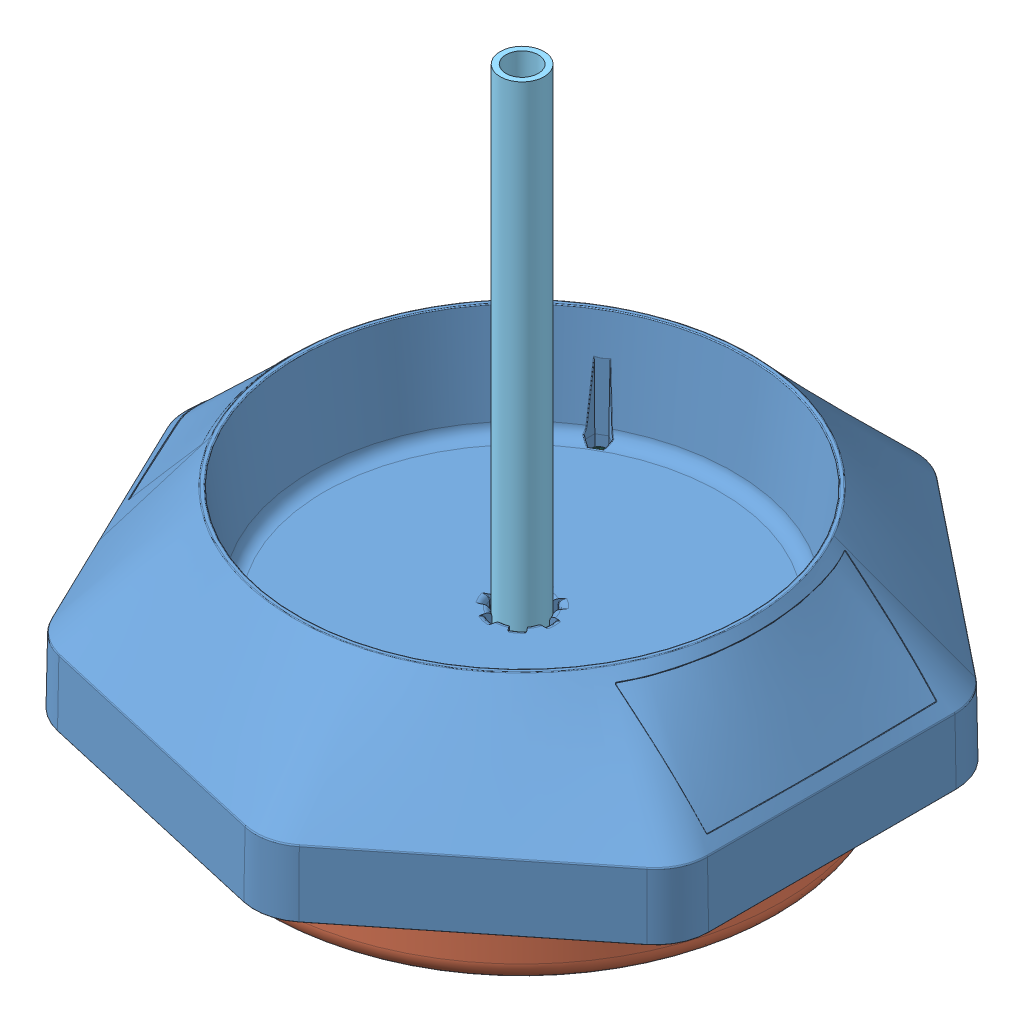
SolidWorks assembly BlueMogo, configuration Default. Lengths in mm.
Overall size (329.62 312.25 329.62).
18 component instances, 8 part files, 0 mates.
Components (placement in the parent):
- BlueMogo.step-1: BlueMogo.step [Default] at origin size (329.62 312.25 329.62)
  - 276-7048-270 Rev3_Red.step-1: 276-7048-270 Rev3_Red.step [Default] x (0 0 -1) z (1 0 0) size (329.62 312.25 329.62)
    - 276-7048-203 Rev5_Yellow.step-1: 276-7048-203 Rev5_Yellow.step [Default] at origin size (322.53 130.15 315.74)
    - 276-7048-204 Rev5.step-1: 276-7048-204 Rev5.step [Default] at (0 -0.25 0) x (-1 0 0) z (0 0 -1) size (260.2 58 260.2)
    - 276-7048-205 Rev1.step-1: 276-7048-205 Rev1.step [Default] at (0 -18.506 0) x (-0.5 0 0.866025) z (0 -1 0) size (241.3 241.3 2)
    - 276-6089-013 Rev4.step-1: 276-6089-013 Rev4.step [Default] at (0 -46.7356 0) x (-0.981976 0 -0.189007) z (0.189007 0 -0.981976) size (60.39 14.6 24.66)
    - 276-6089-013 Rev4.step-2: 276-6089-013 Rev4.step [Default] at (0 -46.7356 0) x (0.981976 0 0.189007) z (-0.189007 0 0.981976) size (60.39 14.6 24.66)
    - 276-7048-209 Rev2.step-1: 276-7048-209 Rev2.step [Default] at (0 101.6 0) x (0.577811 0 0.816171) z (0 1 0) size (21.3 21.3 304.8)
    - 276-1027-001.step-1: 276-1027-001.step [Default] at (-87.9864 15.4 -50.799) x (0.866025 0 -0.5) z (0.5 0 0.866025) size (8.61 5.64 9.94)
    - 276-4999-001 Rev1_No Threads.step-1: 276-4999-001 Rev1_No Threads.step [Default] at (-87.9882 -23.046 -50.8) x (-0.837169 0 -0.546944) z (-0.546944 0 0.837169) size (7.92 46.66 7.92)
    - 276-4993-001 Rev1_No Threads.step-1: 276-4993-001 Rev1_No Threads.step [Default] at (21.0263 -46.7356 8.3751) x (0.527907 -0.843202 0.10161) z (-0.828004 -0.537597 -0.159371) size (7.92 18.09 7.92)
    - 276-1027-001.step-2: 276-1027-001.step [Default] at (87.9864 15.4 -50.799) x (0 0 1) z (-1 0 0) size (8.61 5.64 9.94)
    - 276-1027-001.step-3: 276-1027-001.step [Default] at (0 15.4 101.5979) x (0.866025 0 0.5) z (-0.5 0 0.866025) size (8.61 5.64 9.94)
    - 276-1027-001.step-4: 276-1027-001.step [Default] at (-22.6328 -46.7356 -0.0283) x (0 1 0) z (0.981976 0 0.189007) size (8.61 5.64 9.94)
    - 276-1027-001.step-5: 276-1027-001.step [Default] at (22.6328 -46.7356 0.0283) x (0 1 0) z (-0.981976 0 -0.189007) size (8.61 5.64 9.94)
    - 276-4993-001 Rev1_No Threads.step-2: 276-4993-001 Rev1_No Threads.step [Default] at (-21.0263 -46.7356 -8.3751) x (-0.837157 0.52269 -0.161133) z (-0.513268 -0.852523 -0.098792) size (7.92 18.09 7.92)
    - 276-4999-001 Rev1_No Threads.step-2: 276-4999-001 Rev1_No Threads.step [Default] at (87.9882 -23.046 -50.8) x (-0.925243 0 -0.379375) z (-0.379375 0 0.925243) size (7.92 46.66 7.92)
    - 276-4999-001 Rev1_No Threads.step-3: 276-4999-001 Rev1_No Threads.step [Default] at (0 -23.046 101.6) x (-0.985271 0 -0.170998) z (-0.170998 0 0.985271) size (7.92 46.66 7.92)
